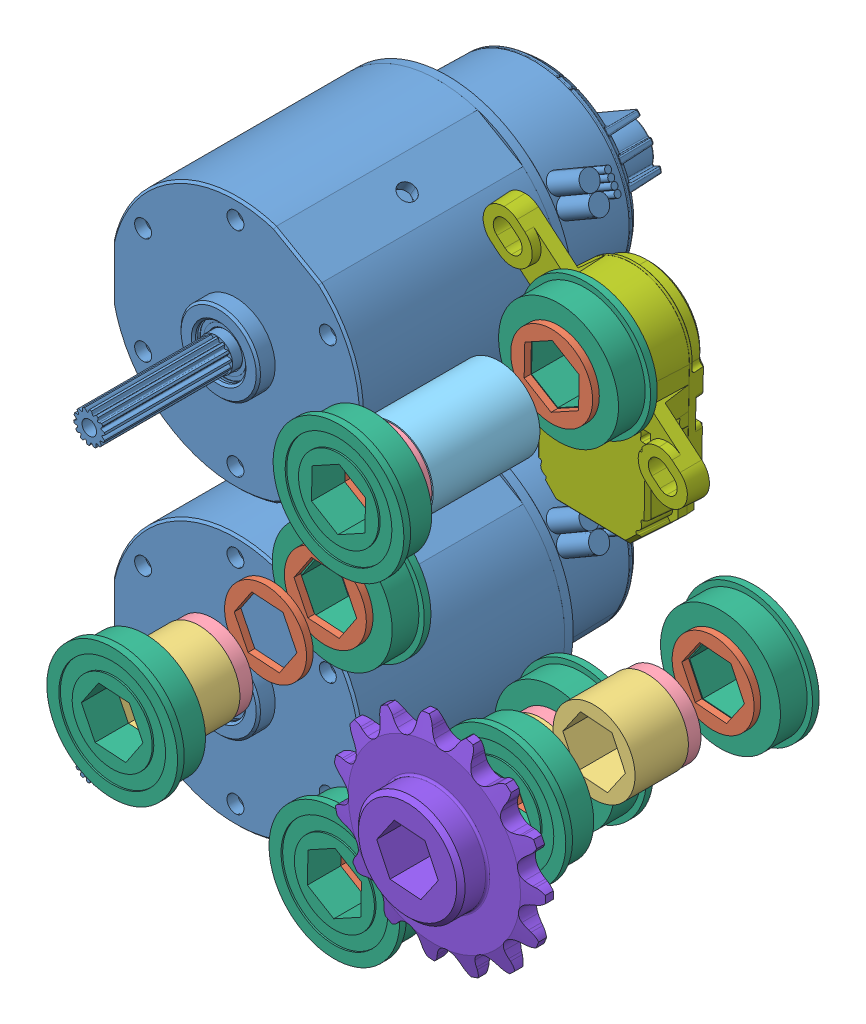
SolidWorks assembly Gearbox, configuration Default. Lengths in mm.
Overall size (196.74 170.26 161.02).
43 component instances, 18 part files, 129 mates.
Components (placement in the parent):
- Falcon500_217-6515-1: Falcon500_217-6515 [Default] at (23.6016 185.8526 207.1038) x (0.866025 -0.5 0) z (0 0 1) size (60 60 115.81)
- Falcon500_217-6515-2: Falcon500_217-6515 [Default] at (23.6016 116.2566 207.1038) x (0.866025 -0.5 0) z (0 0 1) size (60 60 115.81)
- 12T_MotorGear_217-6919.step-1: 12T_MotorGear_217-6919.step [Default] at (23.6016 185.8526 251.5659) x (0.024163 -0.999708 0) z (0 0 1) (suppressed, hidden)
- 12T_MotorGear_217-6919.step-2: 12T_MotorGear_217-6919.step [Default] at (23.6016 116.2566 251.5659) x (-0.668743 0.743494 0) z (0 0 1) (suppressed, hidden)
- 60T_WCP-0121.step-1: 60T_WCP-0121.step [Default] at (52.1675 151.0546 246.8034) x (-0.897339 -0.441342 0) z (0 0 1) (suppressed, hidden)
- 30T_WCP-0706.step-1: 30T_WCP-0706.step [Default] at (105.054 144.0111 275.2768) x (-0.855893 0.517153 0) z (0 0 1) (suppressed, hidden)
- 20T_WCP-0701.step-1: 20T_WCP-0701.step [Default] at (52.1658 151.0292 261.0401) x (0.897339 0.441342 0) z (0 0 1) (suppressed, hidden)
- 64T_WCP-0122.step-1: 64T_WCP-0122.step [Default] at (105.0412 144.0041 261.0401) x (-0.517153 -0.855893 0) z (0 0 1) (suppressed, hidden)
- 54T_WCP-0120.step-1: 54T_WCP-0120.step [Default] at (144.6047 179.8008 275.2895) x (-0.079352 -0.996847 0) z (0 0 1) (suppressed, hidden)
- 20T_WCP-0701.step-2: 20T_WCP-0701.step [Default] at (144.5901 179.802 246.778) x (0.823618 -0.567144 0) z (0 0 1) (suppressed, hidden)
- 72T_WCP-0123.step-1: 72T_WCP-0123.step [Default] at (106.0352 223.693 246.778) x (-0.999802 0.019921 0) z (0 0 1) (suppressed, hidden)
- 6in_Hexshaft_217-4017.step-1: 6in_Hexshaft_217-4017.step [Default] at (52.1658 151.0292 634.5622) x (0.997789 -0.066456 0) z (0 0 1) (suppressed, hidden)
- 6in_Hexshaft_217-4017.step-2: 6in_Hexshaft_217-4017.step [Default] at (105.054 144.0111 634.5622) x (-0.855893 0.517153 0) z (0 0 1) (suppressed, hidden)
- 6in_Hexshaft_217-4017.step-3: 6in_Hexshaft_217-4017.step [Default] at (144.5901 179.802 634.5622) x (-0.567144 -0.823618 0) z (0 0 1) (suppressed, hidden)
- 6in_Hexshaft_217-4017.step-4: 6in_Hexshaft_217-4017.step [Default] at (106.0352 223.693 634.5622) x (0.875814 0.482649 0) z (0 0 1) (suppressed, hidden)
- 0_063_L_500_hex_spacer_217-3257-1: 0_063_L_500_hex_spacer_217-3257 [Default] at (106.0376 223.8103 239.6596) x (0.019921 0.999802 0) z (0 0 1) size (19.5 19.5 1.59)
- 0_063_L_500_hex_spacer_217-3257-2: 0_063_L_500_hex_spacer_217-3257 [Default] at (105.0563 144.1284 268.1584) x (-0.855893 0.517153 0) z (0 0 1) size (19.5 19.5 1.59)
- 0_063_L_500_hex_spacer_217-3257-5: 0_063_L_500_hex_spacer_217-3257 [Default] at (144.4731 179.8113 282.3951) x (-0.567144 -0.823618 0) z (0 0 1) size (19.5 19.5 1.59)
- 0_063_L_500_hex_spacer_217-3257-7: 0_063_L_500_hex_spacer_217-3257 [Default] at (52.1793 151.232 253.9217) x (0.556447 0.830883 0) z (0 0 1) size (19.5 19.5 1.59)
- 0_063_L_500_hex_spacer_217-3257-8: 0_063_L_500_hex_spacer_217-3257 [Default] at (52.1793 151.232 239.685) x (0.556447 0.830883 0) z (0 0 1) size (19.5 19.5 1.59)
- 0_063_L_500_hex_spacer_217-3257-14: 0_063_L_500_hex_spacer_217-3257 [Default] at (105.0563 144.1284 282.3951) x (-0.855893 0.517153 0) z (0 0 1) size (19.5 19.5 1.59)
- 0_063_L_500_hex_spacer_217-3257-23: 0_063_L_500_hex_spacer_217-3257 [Default] at (144.4731 179.8113 239.6596) x (-0.567144 -0.823618 0) z (0 0 1) size (19.5 19.5 1.59)
- 0_063_L_500_hex_spacer_217-3257-25: 0_063_L_500_hex_spacer_217-3257 [Default] at (106.0376 223.8103 282.4713) x (0.019921 0.999802 0) z (0 0 1) size (19.5 19.5 1.59)
- 0_500_L_500_hex_spacer_217-3261-7: 0_500_L_500_hex_spacer_217-3261 [Default] at (144.6566 179.8986 262.6276) x (-0.429702 0.902971 0) z (0 0 1) size (19.5 19.5 12.7)
- 0_500_L_500_hex_spacer_217-3261-8: 0_500_L_500_hex_spacer_217-3261 [Default] at (105.1544 143.9505 248.3655) x (0.875814 0.482649 0) z (0 0 1) size (19.5 19.5 12.7)
- 0_125_L_500_hex_spacer_217-2758-11: 0_125_L_500_hex_spacer_217-2758 [Default] at (144.707 179.7926 254.6901) x (0.079352 0.996847 0) z (0 0 1) size (19.05 19.05 3.17)
- 0_125_L_500_hex_spacer_217-2758-12: 0_125_L_500_hex_spacer_217-2758 [Default] at (105.1568 144.0678 240.428) x (0.517153 0.855893 0) z (0 0 1) size (19.05 19.05 3.17)
- 0_500_L_500_hex_spacer_217-3261-9: 0_500_L_500_hex_spacer_217-3261 [Default] at (52.1523 150.8265 276.8897) x (0.556447 0.830883 0) z (0 0 1) size (19.5 19.5 12.7)
- 0_125_L_500_hex_spacer_217-2758-13: 0_125_L_500_hex_spacer_217-2758 [Default] at (52.2829 151.0214 268.9522) x (0.066456 0.997789 0) z (0 0 1) size (19.05 19.05 3.17)
- 1_000_L_500_hex_spacer_217-3263-1: 1_000_L_500_hex_spacer_217-3263 [Default] at (106.1356 223.6323 265.8026) x (0.875814 0.482649 0) z (0 0 1) size (19.5 19.5 25.4)
- 0_125_L_500_hex_spacer_217-2758-14: 0_125_L_500_hex_spacer_217-2758 [Default] at (106.0329 223.5757 280.0901) x (0.999802 -0.019921 0) z (0 0 1) size (19.05 19.05 3.17)
- 003_Gearbox-1: 003_Gearbox [Default] at (-2.2129 0.5558 286.4401) x (0.999891 -0.014754 0) z (0 0 1) (suppressed, hidden)
- 500ID_1_125OD_Hex_flanged_217-2734-1: 500ID_1_125OD_Hex_flanged_217-2734 [Default] at (106.0376 223.8103 283.2651) x (0.875814 0.482649 0) z (0.482649 -0.875814 0) size (31.12 7.94 31.12)
- 500ID_1_125OD_Hex_flanged_217-2734-2: 500ID_1_125OD_Hex_flanged_217-2734 [Default] at (144.5901 179.802 283.2651) x (0.996847 -0.079352 0) z (-0.079352 -0.996847 0) size (31.12 7.94 31.12)
- 500ID_1_125OD_Hex_flanged_217-2734-3: 500ID_1_125OD_Hex_flanged_217-2734 [Default] at (105.0563 144.1284 283.2651) x (0.875814 0.482649 0) z (0.482649 -0.875814 0) size (31.12 7.94 31.12)
- 500ID_1_125OD_Hex_flanged_217-2734-4: 500ID_1_125OD_Hex_flanged_217-2734 [Default] at (52.1523 150.8265 283.2651) x (0.556447 0.830883 0) z (0.830883 -0.556447 0) size (31.12 7.94 31.12)
- 002_Gearbox-1: 002_Gearbox [Default] at (-2.2129 0.5558 232.4651) x (0.999891 -0.014754 0) z (0 0 1) (suppressed, hidden)
- 500ID_1_125OD_Hex_flanged_217-2734-6: 500ID_1_125OD_Hex_flanged_217-2734 [Default] at (106.0376 223.8103 238.8151) x (0.855893 -0.517153 0) z (0.517153 0.855893 0) size (31.12 7.94 31.12)
- 500ID_1_125OD_Hex_flanged_217-2734-7: 500ID_1_125OD_Hex_flanged_217-2734 [Default] at (144.5901 179.802 238.8151) x (0.996847 -0.079352 0) z (0.079352 0.996847 0) size (31.12 7.94 31.12)
- 500ID_1_125OD_Hex_flanged_217-2734-8: 500ID_1_125OD_Hex_flanged_217-2734 [Default] at (52.1523 150.8265 238.8151) x (0.997789 -0.066456 0) z (0.066456 0.997789 0) size (31.12 7.94 31.12)
- 500ID_1_125OD_Hex_flanged_217-2734-9: 500ID_1_125OD_Hex_flanged_217-2734 [Default] at (105.0563 144.1284 238.8151) x (0.875814 0.482649 0) z (-0.482649 0.875814 0) size (31.12 7.94 31.12)
- REV_Hex_Encoder_REV-11-1271-8: REV_Hex_Encoder_REV-11-1271 [Default] at (106.0396 223.9129 230.4651) x (-0.019152 -0.999817 0) z (0 0 -1) size (57.37 49.78 15.83)
- 15T_#35_500_hex_hubbed_sprocket_217-2660-3: 15T_#35_500_hex_hubbed_sprocket_217-2660 [Default] at (144.5838 179.8152 304.7866) x (0.823618 -0.567144 0) z (0 0 1) size (50.14 50.4 10.67)
Mates (geometry in assembly coordinates):
- Coincident3: coincident aligned: plane of Falcon500_217-6515-1 through (23.6016 185.8526 233.3038) normal (0 0 1); plane of Falcon500_217-6515-2 through (23.6016 116.2566 233.3038) normal (0 0 1)
- Concentric1: concentric aligned: circle of Falcon500_217-6515-1; circle of 12T_MotorGear_217-6919.step-1
- Concentric3: concentric aligned: circle of Falcon500_217-6515-2; circle of 12T_MotorGear_217-6919.step-2
- Distance1: distance = 69.596 mm: point of 12T_MotorGear_217-6919.step-1; point of 12T_MotorGear_217-6919.step-2
- Coincident21: coincident aligned: plane of 60T_WCP-0121.step-1 through (59.5275 150.5644 253.128) normal (-0.830883 0.556447 0); plane of 20T_WCP-0701.step-1 through (55.4148 144.4233 254.7155) normal (-0.830883 0.556447 0)
- Parallel3: parallel aligned: plane of 60T_WCP-0121.step-1 through (52.1675 151.0546 253.128) normal (0 0 1); plane of 20T_WCP-0701.step-1 through (52.1658 151.0292 267.3647) normal (0 0 1)
- Parallel4: parallel aligned: plane of 60T_WCP-0121.step-1 through (52.1675 151.0546 253.128) normal (0 0 1); plane of 20T_WCP-0701.step-1 through (52.1658 151.0292 267.3647) normal (0 0 1)
- Parallel5: parallel aligned: plane of 60T_WCP-0121.step-1 through (48.912 157.6736 253.128) normal (-0.066456 -0.997789 0); plane of 20T_WCP-0701.step-1 through (56.2622 157.1459 254.7155) normal (-0.066456 -0.997789 0)
- Coincident26: coincident aligned: plane of 60T_WCP-0121.step-1 through (48.063 144.9257 253.128) normal (0.897339 0.441342 0); plane of 20T_WCP-0701.step-1 through (44.8204 151.5184 254.7155) normal (0.897339 0.441342 0)
- Coincident28: coincident aligned: plane of 20T_WCP-0701.step-1 through (52.1658 151.0292 267.3647) normal (0 0 1); plane of 64T_WCP-0122.step-1 through (105.0412 144.0041 267.3647) normal (0 0 1)
- Distance11: distance = 45.72 mm: point of 60T_WCP-0121.step-1; point of 12T_MotorGear_217-6919.step-2
- Distance13: distance = 45.72 mm: point of 60T_WCP-0121.step-1; point of 12T_MotorGear_217-6919.step-1
- Distance14: distance = 53.34 mm: point of 64T_WCP-0122.step-1; point of 20T_WCP-0701.step-1
- Coincident34: coincident aligned: plane of 30T_WCP-0706.step-1 through (111.5015 147.5642 268.9522) normal (-0.517153 -0.855893 0); plane of 64T_WCP-0122.step-1 through (105.1881 151.3789 267.3647) normal (-0.517153 -0.855893 0)
- Coincident35: coincident aligned: plane of 30T_WCP-0706.step-1 through (111.3548 140.204 268.9522) normal (-0.999802 0.019921 0); plane of 64T_WCP-0122.step-1 through (111.5015 147.5642 267.3647) normal (-0.999802 0.019921 0)
- Coincident36: coincident aligned: plane of 30T_WCP-0706.step-1 through (105.054 144.0111 281.6014) normal (0 0 1); plane of 54T_WCP-0120.step-1 through (144.6047 179.8008 281.6014) normal (0 0 1)
- Distance15: distance = 53.34 mm: point of 54T_WCP-0120.step-1; point of 30T_WCP-0706.step-1
- Coincident38: coincident aligned: plane of 54T_WCP-0120.step-1 through (137.2516 180.3861 268.9776) normal (0.902971 0.429702 0); plane of 20T_WCP-0701.step-2 through (137.2516 180.3861 240.4534) normal (0.902971 0.429702 0)
- Coincident39: coincident aligned: plane of 54T_WCP-0120.step-1 through (141.4351 186.4614 268.9776) normal (0.823618 -0.567144 0); plane of 20T_WCP-0701.step-2 through (141.4267 186.4493 240.4534) normal (0.823618 -0.567144 0)
- Coincident40: coincident aligned: plane of 20T_WCP-0701.step-2 through (144.5901 179.802 240.4534) normal (0 0 -1); plane of 72T_WCP-0123.step-1 through (106.0352 223.693 240.4534) normal (0 0 -1)
- Distance16: distance = 58.42 mm: point of 72T_WCP-0123.step-1; point of 20T_WCP-0701.step-2
- Concentric4: concentric anti-aligned: circle of 20T_WCP-0701.step-1; circle of 6in_Hexshaft_217-4017.step-1
- Parallel14: parallel anti-aligned: plane of 20T_WCP-0701.step-1 through (56.2622 157.1459 254.7155) normal (-0.066456 -0.997789 0); plane of 6in_Hexshaft_217-4017.step-1 through (56.2622 157.1459 1091.7622) normal (0.066456 0.997789 0)
- Concentric5: concentric anti-aligned: circle of 30T_WCP-0706.step-1; circle of 6in_Hexshaft_217-4017.step-2
- Parallel13: parallel anti-aligned: plane of 30T_WCP-0706.step-1 through (98.7532 147.8183 268.9522) normal (0.999802 -0.019921 0); plane of 6in_Hexshaft_217-4017.step-2 through (98.7532 147.8183 1091.7622) normal (-0.999802 0.019921 0)
- Concentric6: concentric anti-aligned: circle of 20T_WCP-0701.step-2; circle of 6in_Hexshaft_217-4017.step-3
- Parallel12: parallel anti-aligned: plane of 20T_WCP-0701.step-2 through (141.4267 186.4493 240.4534) normal (0.823618 -0.567144 0); plane of 6in_Hexshaft_217-4017.step-3 through (141.4267 186.4493 1091.7622) normal (-0.823618 0.567144 0)
- Concentric7: concentric anti-aligned: circle of 72T_WCP-0123.step-1; circle of 6in_Hexshaft_217-4017.step-4
- Parallel11: parallel anti-aligned: plane of 72T_WCP-0123.step-1 through (105.8883 216.3181 253.1026) normal (0.517153 0.855893 0); plane of 6in_Hexshaft_217-4017.step-4 through (99.5878 220.1399 1091.7622) normal (-0.517153 -0.855893 0)
- Coincident41: coincident aligned: plane of 20T_WCP-0701.step-1 through (52.1658 151.0292 267.3647) normal (0 0 1); plane of 64T_WCP-0122.step-1 through (105.0412 144.0041 267.3647) normal (0 0 1)
- Coincident54: coincident aligned: plane of 12T_MotorGear_217-6919.step-1 through (23.6016 185.8526 261.0909) normal (0 0 1); plane of 12T_MotorGear_217-6919.step-2 through (23.6016 116.2566 261.0909) normal (0 0 1)
- Coincident133: coincident aligned: plane of 12T_MotorGear_217-6919.step-1 through (23.6016 185.8526 242.0409) normal (0 0 -1); plane of 60T_WCP-0121.step-1 through (69.5431 115.7263 242.0409) normal (0 0 -1)
- Distance19: distance = 3.175 mm anti-aligned: plane of 60T_WCP-0121.step-1 through (52.1675 151.0546 240.4788) normal (0 0 -1); plane of Falcon500_217-6515-1 through (23.6016 185.8526 237.3038) normal (0 0 1)
- Coincident186: coincident aligned: plane of 6in_Hexshaft_217-4017.step-2 through (105.054 144.0111 329.7622) normal (0 0 1); plane of 6in_Hexshaft_217-4017.step-4 through (106.0352 223.693 329.7622) normal (0 0 1)
- Coincident187: coincident aligned: plane of 6in_Hexshaft_217-4017.step-1 through (52.1658 151.0292 329.7622) normal (0 0 1); plane of 6in_Hexshaft_217-4017.step-3 through (144.5901 179.802 329.7622) normal (0 0 1)
- Coincident188: coincident aligned: plane of 6in_Hexshaft_217-4017.step-2 through (105.054 144.0111 329.7622) normal (0 0 1); plane of 6in_Hexshaft_217-4017.step-3 through (144.5901 179.802 329.7622) normal (0 0 1)
- Coincident189: coincident anti-aligned: plane of 6in_Hexshaft_217-4017.step-4 through (99.5878 220.1399 1091.7622) normal (-0.517153 -0.855893 0); plane of 0_063_L_500_hex_spacer_217-3257-1 through (99.4874 220.2005 240.4534) normal (0.517153 0.855893 0)
- Coincident190: coincident anti-aligned: plane of 6in_Hexshaft_217-4017.step-4 through (105.8886 216.3327 1091.7622) normal (0.482649 -0.875814 0); plane of 0_063_L_500_hex_spacer_217-3257-1 through (105.8886 216.3327 240.4534) normal (-0.482649 0.875814 0)
- Coincident193: coincident anti-aligned: plane of 6in_Hexshaft_217-4017.step-2 through (98.6065 140.458 1091.7622) normal (-0.517153 -0.855893 0); plane of 0_063_L_500_hex_spacer_217-3257-2 through (98.5061 140.5187 268.9522) normal (0.517153 0.855893 0)
- Coincident194: coincident anti-aligned: plane of 6in_Hexshaft_217-4017.step-2 through (104.9074 136.6509 1091.7622) normal (0.482649 -0.875814 0); plane of 0_063_L_500_hex_spacer_217-3257-2 through (104.9074 136.6509 268.9522) normal (-0.482649 0.875814 0)
- Coincident201: coincident anti-aligned: plane of 6in_Hexshaft_217-4017.step-3 through (151.9285 179.2178 1091.7622) normal (0.902971 0.429702 0); plane of 0_063_L_500_hex_spacer_217-3257-5 through (151.9285 179.2178 283.1889) normal (-0.902971 -0.429702 0)
- Coincident202: coincident anti-aligned: plane of 6in_Hexshaft_217-4017.step-3 through (147.7534 173.1546 1091.7622) normal (0.823618 -0.567144 0); plane of 0_063_L_500_hex_spacer_217-3257-5 through (147.6869 173.058 283.1889) normal (-0.823618 0.567144 0)
- Coincident205: coincident anti-aligned: plane of 6in_Hexshaft_217-4017.step-1 through (44.8204 151.5184 1091.7622) normal (-0.897339 -0.441342 0); plane of 0_063_L_500_hex_spacer_217-3257-7 through (44.7169 151.729 254.7155) normal (0.897339 0.441342 0)
- Coincident206: coincident anti-aligned: plane of 6in_Hexshaft_217-4017.step-1 through (55.4148 144.4233 1091.7622) normal (0.830883 -0.556447 0); plane of 0_063_L_500_hex_spacer_217-3257-7 through (55.4801 144.5208 254.7155) normal (-0.830883 0.556447 0)
- Coincident207: coincident anti-aligned: plane of 6in_Hexshaft_217-4017.step-1 through (44.8204 151.5184 1091.7622) normal (-0.897339 -0.441342 0); plane of 0_063_L_500_hex_spacer_217-3257-8 through (44.7169 151.729 240.4788) normal (0.897339 0.441342 0)
- Coincident208: coincident anti-aligned: plane of 6in_Hexshaft_217-4017.step-1 through (55.4148 144.4233 1091.7622) normal (0.830883 -0.556447 0); plane of 0_063_L_500_hex_spacer_217-3257-8 through (55.4801 144.5208 240.4788) normal (-0.830883 0.556447 0)
- Coincident219: coincident anti-aligned: plane of 6in_Hexshaft_217-4017.step-2 through (98.6065 140.458 1091.7622) normal (-0.517153 -0.855893 0); plane of 0_063_L_500_hex_spacer_217-3257-14 through (98.5061 140.5187 283.1889) normal (0.517153 0.855893 0)
- Coincident220: coincident anti-aligned: plane of 6in_Hexshaft_217-4017.step-2 through (104.9074 136.6509 1091.7622) normal (0.482649 -0.875814 0); plane of 0_063_L_500_hex_spacer_217-3257-14 through (104.9074 136.6509 283.1889) normal (-0.482649 0.875814 0)
- Coincident237: coincident anti-aligned: plane of 6in_Hexshaft_217-4017.step-3 through (151.9285 179.2178 1091.7622) normal (0.902971 0.429702 0); plane of 0_063_L_500_hex_spacer_217-3257-23 through (151.9285 179.2178 240.4534) normal (-0.902971 -0.429702 0)
- Coincident238: coincident anti-aligned: plane of 6in_Hexshaft_217-4017.step-3 through (147.7534 173.1546 1091.7622) normal (0.823618 -0.567144 0); plane of 0_063_L_500_hex_spacer_217-3257-23 through (147.6869 173.058 240.4534) normal (-0.823618 0.567144 0)
- Coincident241: coincident anti-aligned: plane of 6in_Hexshaft_217-4017.step-4 through (99.5878 220.1399 1091.7622) normal (-0.517153 -0.855893 0); plane of 0_063_L_500_hex_spacer_217-3257-25 through (99.4874 220.2005 283.2651) normal (0.517153 0.855893 0)
- Coincident242: coincident anti-aligned: plane of 6in_Hexshaft_217-4017.step-4 through (105.8886 216.3327 1091.7622) normal (0.482649 -0.875814 0); plane of 0_063_L_500_hex_spacer_217-3257-25 through (105.8886 216.3327 283.2651) normal (-0.482649 0.875814 0)
- Coincident255: coincident anti-aligned: plane of 60T_WCP-0121.step-1 through (52.1675 151.0546 253.128) normal (0 0 1); plane of 0_063_L_500_hex_spacer_217-3257-7 through (52.1793 151.232 253.128) normal (0 0 -1)
- Coincident256: coincident anti-aligned: plane of 20T_WCP-0701.step-1 through (52.1658 151.0292 254.7155) normal (0 0 -1); plane of 0_063_L_500_hex_spacer_217-3257-7 through (52.1793 151.232 254.7155) normal (0 0 1)
- Coincident257: coincident anti-aligned: plane of 64T_WCP-0122.step-1 through (105.0412 144.0041 267.3647) normal (0 0 1); plane of 0_063_L_500_hex_spacer_217-3257-2 through (105.0563 144.1284 267.3647) normal (0 0 -1)
- Coincident258: coincident anti-aligned: plane of 30T_WCP-0706.step-1 through (105.054 144.0111 268.9522) normal (0 0 -1); plane of 0_063_L_500_hex_spacer_217-3257-2 through (105.0563 144.1284 268.9522) normal (0 0 1)
- Coincident259: coincident anti-aligned: plane of 54T_WCP-0120.step-1 through (144.6047 179.8008 281.6014) normal (0 0 1); plane of 0_063_L_500_hex_spacer_217-3257-5 through (144.4731 179.8113 281.6014) normal (0 0 -1)
- Coincident260: coincident anti-aligned: plane of 6in_Hexshaft_217-4017.step-3 through (140.4149 173.7387 1091.7622) normal (-0.079352 -0.996847 0); plane of 0_500_L_500_hex_spacer_217-3261-7 through (140.4149 173.7387 268.9776) normal (0.079352 0.996847 0)
- Coincident261: coincident anti-aligned: plane of 6in_Hexshaft_217-4017.step-3 through (137.2516 180.3861 1091.7622) normal (-0.902971 -0.429702 0); plane of 0_500_L_500_hex_spacer_217-3261-7 through (137.2012 180.4921 268.9776) normal (0.902971 0.429702 0)
- Coincident262: coincident aligned: circle of 54T_WCP-0120.step-1; plane of 0_500_L_500_hex_spacer_217-3261-7 through (144.6566 179.8986 268.9776) normal (0 0 1)
- Coincident263: coincident anti-aligned: plane of 6in_Hexshaft_217-4017.step-3 through (137.2516 180.3861 1091.7622) normal (-0.902971 -0.429702 0); plane of 0_125_L_500_hex_spacer_217-2758-11 through (137.2516 180.3861 256.2776) normal (0.902971 0.429702 0)
- Coincident264: coincident anti-aligned: plane of 6in_Hexshaft_217-4017.step-3 through (141.4267 186.4493 1091.7622) normal (-0.823618 0.567144 0); plane of 0_125_L_500_hex_spacer_217-2758-11 through (141.4933 186.546 256.2776) normal (0.823618 -0.567144 0)
- Coincident265: coincident anti-aligned: plane of 0_125_L_500_hex_spacer_217-2758-11 through (144.707 179.7926 256.2776) normal (0 0 1); plane of 0_500_L_500_hex_spacer_217-3261-7 through (144.6566 179.8986 256.2776) normal (0 0 -1)
- Coincident266: coincident anti-aligned: plane of 20T_WCP-0701.step-2 through (144.5901 179.802 253.1026) normal (0 0 1); plane of 0_125_L_500_hex_spacer_217-2758-11 through (144.707 179.7926 253.1026) normal (0 0 -1)
- Coincident267: coincident anti-aligned: plane of 72T_WCP-0123.step-1 through (106.0352 223.693 240.4534) normal (0 0 -1); plane of 0_063_L_500_hex_spacer_217-3257-1 through (106.0376 223.8103 240.4534) normal (0 0 1)
- Coincident268: coincident anti-aligned: plane of 20T_WCP-0701.step-2 through (144.5901 179.802 240.4534) normal (0 0 -1); plane of 0_063_L_500_hex_spacer_217-3257-23 through (144.4731 179.8113 240.4534) normal (0 0 1)
- Coincident269: coincident anti-aligned: plane of 30T_WCP-0706.step-1 through (105.054 144.0111 281.6014) normal (0 0 1); plane of 0_063_L_500_hex_spacer_217-3257-14 through (105.0563 144.1284 281.6014) normal (0 0 -1)
- Coincident270: coincident anti-aligned: plane of 6in_Hexshaft_217-4017.step-2 through (98.7532 147.8183 1091.7622) normal (-0.999802 0.019921 0); plane of 0_500_L_500_hex_spacer_217-3261-8 through (98.7532 147.8183 254.7155) normal (0.999802 -0.019921 0)
- Coincident271: coincident anti-aligned: plane of 6in_Hexshaft_217-4017.step-2 through (105.2007 151.3714 1091.7622) normal (-0.482649 0.875814 0); plane of 0_500_L_500_hex_spacer_217-3261-8 through (105.3034 151.428 254.7155) normal (0.482649 -0.875814 0)
- Coincident272: coincident anti-aligned: plane of 64T_WCP-0122.step-1 through (105.0412 144.0041 254.7155) normal (0 0 -1); plane of 0_500_L_500_hex_spacer_217-3261-8 through (105.1544 143.9505 254.7155) normal (0 0 1)
- Coincident273: coincident anti-aligned: plane of 6in_Hexshaft_217-4017.step-2 through (98.6065 140.458 1091.7622) normal (-0.517153 -0.855893 0); plane of 0_125_L_500_hex_spacer_217-2758-12 through (98.6065 140.458 242.0155) normal (0.517153 0.855893 0)
- Coincident274: coincident anti-aligned: plane of 6in_Hexshaft_217-4017.step-2 through (98.7532 147.8183 1091.7622) normal (-0.999802 0.019921 0); plane of 0_125_L_500_hex_spacer_217-2758-12 through (98.7555 147.9355 242.0155) normal (0.999802 -0.019921 0)
- Coincident275: coincident anti-aligned: plane of 0_500_L_500_hex_spacer_217-3261-8 through (105.1544 143.9505 242.0155) normal (0 0 -1); plane of 0_125_L_500_hex_spacer_217-2758-12 through (105.1568 144.0678 242.0155) normal (0 0 1)
- Coincident276: coincident anti-aligned: plane of 60T_WCP-0121.step-1 through (52.1675 151.0546 240.4788) normal (0 0 -1); plane of 0_063_L_500_hex_spacer_217-3257-8 through (52.1793 151.232 240.4788) normal (0 0 1)
- Coincident277: coincident anti-aligned: plane of 6in_Hexshaft_217-4017.step-1 through (48.9168 157.6351 1091.7622) normal (-0.830883 0.556447 0); plane of 0_125_L_500_hex_spacer_217-2758-13 through (48.9821 157.7326 270.5397) normal (0.830883 -0.556447 0)
- Coincident278: coincident anti-aligned: plane of 6in_Hexshaft_217-4017.step-1 through (44.8204 151.5184 1091.7622) normal (-0.897339 -0.441342 0); plane of 0_125_L_500_hex_spacer_217-2758-13 through (44.8204 151.5184 270.5397) normal (0.897339 0.441342 0)
- Coincident279: coincident anti-aligned: plane of 20T_WCP-0701.step-1 through (52.1658 151.0292 267.3647) normal (0 0 1); plane of 0_125_L_500_hex_spacer_217-2758-13 through (52.2829 151.0214 267.3647) normal (0 0 -1)
- Coincident280: coincident anti-aligned: plane of 6in_Hexshaft_217-4017.step-1 through (48.9168 157.6351 1091.7622) normal (-0.830883 0.556447 0); plane of 0_500_L_500_hex_spacer_217-3261-9 through (48.8515 157.5377 283.2397) normal (0.830883 -0.556447 0)
- Coincident281: coincident anti-aligned: plane of 6in_Hexshaft_217-4017.step-1 through (59.5112 150.54 1091.7622) normal (0.897339 0.441342 0); plane of 0_500_L_500_hex_spacer_217-3261-9 through (59.6148 150.3295 283.2397) normal (-0.897339 -0.441342 0)
- Coincident282: coincident anti-aligned: plane of 0_500_L_500_hex_spacer_217-3261-9 through (52.1523 150.8265 270.5397) normal (0 0 -1); plane of 0_125_L_500_hex_spacer_217-2758-13 through (52.2829 151.0214 270.5397) normal (0 0 1)
- Coincident283: coincident anti-aligned: plane of 6in_Hexshaft_217-4017.step-4 through (99.7344 227.5001 1091.7622) normal (-0.999802 0.019921 0); plane of 1_000_L_500_hex_spacer_217-3263-1 through (99.7344 227.5001 278.5026) normal (0.999802 -0.019921 0)
- Coincident284: coincident anti-aligned: plane of 6in_Hexshaft_217-4017.step-4 through (106.1819 231.0532 1091.7622) normal (-0.482649 0.875814 0); plane of 1_000_L_500_hex_spacer_217-3263-1 through (106.2846 231.1098 278.5026) normal (0.482649 -0.875814 0)
- Coincident285: coincident anti-aligned: plane of 72T_WCP-0123.step-1 through (106.0352 223.693 253.1026) normal (0 0 1); plane of 1_000_L_500_hex_spacer_217-3263-1 through (106.1356 223.6323 253.1026) normal (0 0 -1)
- Coincident286: coincident anti-aligned: plane of 6in_Hexshaft_217-4017.step-4 through (112.4827 227.2461 1091.7622) normal (0.517153 0.855893 0); plane of 0_125_L_500_hex_spacer_217-2758-14 through (112.5831 227.1854 281.6776) normal (-0.517153 -0.855893 0)
- Coincident287: coincident anti-aligned: plane of 6in_Hexshaft_217-4017.step-4 through (106.1819 231.0532 1091.7622) normal (-0.482649 0.875814 0); plane of 0_125_L_500_hex_spacer_217-2758-14 through (106.1819 231.0532 281.6776) normal (0.482649 -0.875814 0)
- Coincident288: coincident anti-aligned: plane of 1_000_L_500_hex_spacer_217-3263-1 through (106.1356 223.6323 278.5026) normal (0 0 1); plane of 0_125_L_500_hex_spacer_217-2758-14 through (106.0329 223.5757 278.5026) normal (0 0 -1)
- Coincident289: coincident anti-aligned: plane of 0_063_L_500_hex_spacer_217-3257-25 through (106.0376 223.8103 281.6776) normal (0 0 -1); plane of 0_125_L_500_hex_spacer_217-2758-14 through (106.0329 223.5757 281.6776) normal (0 0 1)
- Coincident290: coincident aligned: plane of Falcon500_217-6515-1 through (23.6016 185.8526 268.1063) normal (0 0 1); plane of Falcon500_217-6515-2 through (23.6016 116.2566 268.1063) normal (0 0 1)
- Coincident291: coincident aligned: plane of Falcon500_217-6515-1 through (-5.7401 185.8526 229.3038) normal (-1 0 0); plane of Falcon500_217-6515-2 through (-5.7401 116.2566 229.3038) normal (-1 0 0)
- Concentric8: concentric aligned: circle of 6in_Hexshaft_217-4017.step-3; circle of 003_Gearbox-1
- Concentric11: concentric anti-aligned: circle of 0_063_L_500_hex_spacer_217-3257-25; circle of 003_Gearbox-1
- Concentric12: concentric anti-aligned: circle of 0_063_L_500_hex_spacer_217-3257-14; circle of 003_Gearbox-1
- Concentric13: concentric anti-aligned: circle of 0_500_L_500_hex_spacer_217-3261-9; circle of 003_Gearbox-1
- Coincident300: coincident anti-aligned: plane of 003_Gearbox-1 through (-2.2129 0.5558 289.6151) normal (0 0 1); plane of 500ID_1_125OD_Hex_flanged_217-2734-1 through (119.663 231.3191 289.6151) normal (0 0 -1)
- Concentric14: concentric anti-aligned: circle of 003_Gearbox-1; circle of 500ID_1_125OD_Hex_flanged_217-2734-1
- Parallel16: parallel anti-aligned: plane of 6in_Hexshaft_217-4017.step-4 through (106.1819 231.0532 1091.7622) normal (-0.482649 0.875814 0); plane of 500ID_1_125OD_Hex_flanged_217-2734-1 through (106.1839 231.1527 283.2651) normal (0.482649 -0.875814 0)
- Coincident303: coincident anti-aligned: plane of 0_063_L_500_hex_spacer_217-3257-25 through (106.0376 223.8103 283.2651) normal (0 0 1); plane of 500ID_1_125OD_Hex_flanged_217-2734-1 through (118.5396 230.7 283.2651) normal (0 0 -1)
- Coincident304: coincident anti-aligned: plane of 003_Gearbox-1 through (-2.2129 0.5558 289.6151) normal (0 0 1); plane of 500ID_1_125OD_Hex_flanged_217-2734-2 through (160.0985 178.5674 289.6151) normal (0 0 -1)
- Coincident305: coincident anti-aligned: plane of 003_Gearbox-1 through (-2.2129 0.5558 289.6151) normal (0 0 1); plane of 500ID_1_125OD_Hex_flanged_217-2734-3 through (118.6818 151.6372 289.6151) normal (0 0 -1)
- Coincident306: coincident anti-aligned: plane of 003_Gearbox-1 through (-2.2129 0.5558 289.6151) normal (0 0 1); plane of 500ID_1_125OD_Hex_flanged_217-2734-4 through (60.8092 163.7529 289.6151) normal (0 0 -1)
- Concentric16: concentric anti-aligned: circle of 003_Gearbox-1; circle of 500ID_1_125OD_Hex_flanged_217-2734-2
- Parallel18: parallel anti-aligned: plane of 6in_Hexshaft_217-4017.step-3 through (148.7652 185.8652 1091.7622) normal (0.079352 0.996847 0); plane of 500ID_1_125OD_Hex_flanged_217-2734-2 through (148.7551 185.8505 283.2651) normal (-0.079352 -0.996847 0)
- Concentric17: concentric anti-aligned: circle of 003_Gearbox-1; circle of 500ID_1_125OD_Hex_flanged_217-2734-3
- Parallel19: parallel anti-aligned: plane of 6in_Hexshaft_217-4017.step-2 through (105.2007 151.3714 1091.7622) normal (-0.482649 0.875814 0); plane of 500ID_1_125OD_Hex_flanged_217-2734-3 through (105.2026 151.4709 283.2651) normal (0.482649 -0.875814 0)
- Concentric18: concentric anti-aligned: circle of 003_Gearbox-1; circle of 500ID_1_125OD_Hex_flanged_217-2734-4
- Parallel20: parallel anti-aligned: plane of 6in_Hexshaft_217-4017.step-1 through (48.9168 157.6351 1091.7622) normal (-0.830883 0.556447 0); plane of 500ID_1_125OD_Hex_flanged_217-2734-4 through (48.9111 157.4164 283.2651) normal (0.830883 -0.556447 0)
- Coincident320: coincident anti-aligned: plane of 002_Gearbox-1 through (-2.2129 0.5558 232.4651) normal (0 0 -1); plane of 500ID_1_125OD_Hex_flanged_217-2734-6 through (119.3531 215.7647 232.4651) normal (0 0 1)
- Coincident321: coincident anti-aligned: plane of 002_Gearbox-1 through (-2.2129 0.5558 232.4651) normal (0 0 -1); plane of 500ID_1_125OD_Hex_flanged_217-2734-7 through (160.0985 178.5674 232.4651) normal (0 0 1)
- Coincident322: coincident anti-aligned: plane of 002_Gearbox-1 through (-2.2129 0.5558 232.4651) normal (0 0 -1); plane of 500ID_1_125OD_Hex_flanged_217-2734-8 through (67.6754 149.7926 232.4651) normal (0 0 1)
- Coincident323: coincident anti-aligned: plane of 002_Gearbox-1 through (-2.2129 0.5558 232.4651) normal (0 0 -1); plane of 500ID_1_125OD_Hex_flanged_217-2734-9 through (118.6818 151.6372 232.4651) normal (0 0 1)
- Concentric20: concentric aligned: circle of 002_Gearbox-1; circle of 500ID_1_125OD_Hex_flanged_217-2734-6
- Concentric21: concentric aligned: circle of 002_Gearbox-1; circle of 500ID_1_125OD_Hex_flanged_217-2734-7
- Concentric22: concentric aligned: circle of 002_Gearbox-1; circle of 500ID_1_125OD_Hex_flanged_217-2734-9
- Concentric23: concentric aligned: circle of 002_Gearbox-1; circle of 500ID_1_125OD_Hex_flanged_217-2734-8
- Parallel21: parallel anti-aligned: plane of 6in_Hexshaft_217-4017.step-2 through (105.2007 151.3714 1091.7622) normal (-0.482649 0.875814 0); plane of 500ID_1_125OD_Hex_flanged_217-2734-9 through (98.7708 147.9264 238.8151) normal (0.482649 -0.875814 0)
- Parallel22: parallel anti-aligned: plane of 6in_Hexshaft_217-4017.step-3 through (148.7652 185.8652 1091.7622) normal (0.079352 0.996847 0); plane of 500ID_1_125OD_Hex_flanged_217-2734-7 through (141.4344 186.4333 238.8151) normal (-0.079352 -0.996847 0)
- Parallel23: parallel anti-aligned: plane of 6in_Hexshaft_217-4017.step-4 through (106.1819 231.0532 1091.7622) normal (-0.482649 0.875814 0); plane of 500ID_1_125OD_Hex_flanged_217-2734-6 through (99.752 227.6082 238.8151) normal (0.482649 -0.875814 0)
- Parallel24: parallel anti-aligned: plane of 6in_Hexshaft_217-4017.step-1 through (48.9168 157.6351 1091.7622) normal (-0.830883 0.556447 0); plane of 500ID_1_125OD_Hex_flanged_217-2734-8 through (44.8246 151.3145 238.8151) normal (0.830883 -0.556447 0)
- Distance20: distance = 50.8 mm anti-aligned: plane of 003_Gearbox-1 through (-2.2129 0.5558 286.4401) normal (0 0 -1); plane of 002_Gearbox-1 through (-2.2129 0.5558 235.6401) normal (0 0 1)
- Coincident340: coincident aligned: plane of 003_Gearbox-1 through (1.8454 275.5862 289.6151) normal (0.014754 0.999891 0); plane of 002_Gearbox-1 through (-60.1826 276.5015 235.6401) normal (0.014754 0.999891 0)
- Coincident341: coincident aligned: plane of 003_Gearbox-1 through (269.9009 95.0743 289.6151) normal (0.944637 0.328119 0); plane of 002_Gearbox-1 through (208.2582 272.5404 235.6401) normal (0.944637 0.328119 0)
- Coincident342: coincident aligned: plane of 003_Gearbox-1 through (-0.9653 85.1069 289.6151) normal (-0.014754 -0.999891 0); plane of 002_Gearbox-1 through (241.7736 81.5251 235.6401) normal (-0.014754 -0.999891 0)
- Coincident343: coincident aligned: plane of 003_Gearbox-1 through (-64.2409 1.4711 289.6151) normal (-0.999891 0.014754 0); plane of 002_Gearbox-1 through (-62.9933 86.0222 235.6401) normal (-0.999891 0.014754 0)
- Parallel26: parallel anti-aligned: plane of 002_Gearbox-1 through (-2.2129 0.5558 232.4651) normal (0 0 -1); plane of REV_Hex_Encoder_REV-11-1271-8 through (106.0396 223.9129 230.4651) normal (0 0 1)
- Coincident350: coincident anti-aligned: plane of 002_Gearbox-1 through (-2.2129 0.5558 232.4651) normal (0 0 -1); plane of REV_Hex_Encoder_REV-11-1271-8 through (86.6178 240.2821 232.4651) normal (0 0 1)
- Concentric24: concentric anti-aligned: circle of 002_Gearbox-1; circle of REV_Hex_Encoder_REV-11-1271-8
- Coincident352: coincident anti-aligned: cylinder of 002_Gearbox-1; cylinder of REV_Hex_Encoder_REV-11-1271-8 through (125.4615 207.5437 232.4651) axis (0 0 -1) radius 2.4892
- Coincident353: coincident anti-aligned: plane of 6in_Hexshaft_217-4017.step-3 through (141.4267 186.4493 1091.7622) normal (-0.823618 0.567144 0); plane of 15T_#35_500_hex_hubbed_sprocket_217-2660-3 through (141.4267 186.4493 313.3157) normal (0.823618 -0.567144 0)
- Coincident355: coincident anti-aligned: plane of 6in_Hexshaft_217-4017.step-3 through (148.7652 185.8652 1091.7622) normal (0.079352 0.996847 0); plane of 15T_#35_500_hex_hubbed_sprocket_217-2660-3 through (148.7506 185.8663 313.3157) normal (-0.079352 -0.996847 0)
